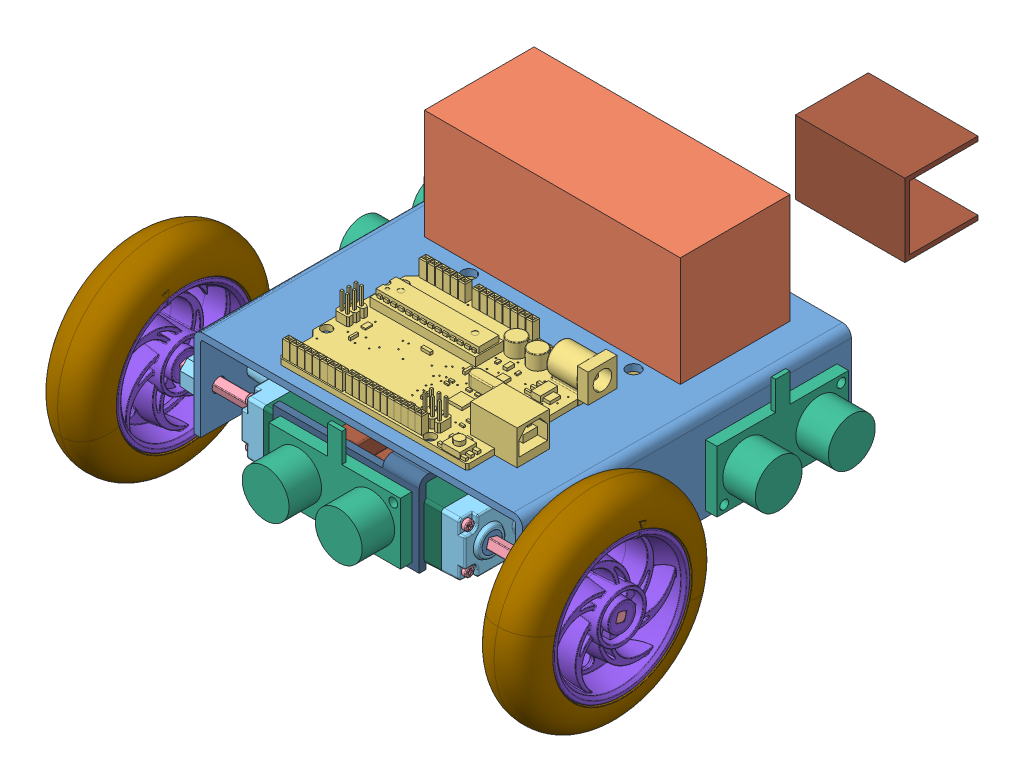
SolidWorks assembly mte380_Assy_02_minibot_01, configuration Default. Lengths in mm.
Overall size (174.7 100.24 233.03).
81 component instances, 29 part files, 49 mates.
Components (placement in the parent):
- mte380_02_frame_02-1: mte380_02_frame_02 [Default] at (-259.485 58.7791 95.25) size (114.15 31.84 114.3)
- mte380_02_package_01-1: mte380_02_package_01 [Default] at (-218.21 58.7791 46.8312) size (88.9 38.1 38.1)
- Arduino_Predeterminado-1: Arduino_Predeterminado [Default] at (-170.1744 58.7791 84.8989) x (-0.999979 0 0.006548) z (-0.006548 0 -0.999979) size (75 12 51.02)
- mte380_01_vex_motor_269-1: mte380_01_vex_motor_269 [Default] at (-184.6716 39.6426 96.8201) x (0 0 1) z (1 0 0) size (46.4 20.59 51.86)
  - SPPM206-0150BO-1: SPPM206-0150BO [Default] at (17.3 7.3 -1.5) x (1 0 0) z (0 -1 0) size (3.3 16.36 3.3)
  - 276-2181-003 Rev1-1: 276-2181-003 Rev1 [Default] at (0 0 -28) size (38.95 18.95 25.5)
  - 276-2177-019 Rev1-1: 276-2177-019 Rev1 [Default] at (-14.2702 0 -28) x (0.144195 -0.989549 0) z (0.989549 0.144195 0) size (6.3 15.8 6.3)
  - 276-2181-011 Rev1-1: 276-2181-011 Rev1 [Default] at (11.1298 0 -11) x (-1 0 0) z (0 1 0) size (11 4 11)
  - QFK-N30QAV-16068-1: QFK-N30QAV-16068 [Default] at (-12.9 0 -23) x (0 1 0) z (0 0 1) size (12 10 26.1)
  - SPPM143-0030BO-1: SPPM143-0030BO [Default] at (-12.9 4.25 -6) x (-1 0 0) z (0 1 0) size (2.4 6.08 2.4)
  - 276-2181-010 Rev1-1: 276-2181-010 Rev1 [Default] at (10.8763 0 -9.4) x (0.878827 0.47714 0) z (0 0 1) size (1.5 1.5 16)
  - 276-2181-001 Rev1-1: 276-2181-001 Rev1 [Default] at origin size (40 20 8.06)
  - 276-2181-006 Rev1-1: 276-2181-006 Rev1 [Default] at (10.8763 0 -1.05) x (-0.259931 -0.965627 0) z (0 0 1) size (14.22 14.25 6.9)
  - 276-2181-007 Rev1-1: 276-2181-007 Rev1 [Default] at (2.1533 -1.4937 -4.4) x (-0.202497 0.979283 0) z (0 0 1) size (14.22 14.25 14.9)
  - 276-2181-010 Rev1-2: 276-2181-010 Rev1 [Default] at (-5.7003 2.586 -9.4) size (1.5 1.5 16)
  - 276-2177-018 Rev1-1: 276-2177-018 Rev1 [Default] at (-18.5 0.1 2.5) x (0 1 0) z (1 0 0) size (6.4 4.2 8.9)
  - 276-2181-006 Rev1-2: 276-2181-006 Rev1 [Default] at (2.1533 -1.4937 2.75) x (-0.071378 0.997449 0) z (0 0 1) size (14.22 14.25 6.9)
  - 276-2181-002 Rev1-1: 276-2181-002 Rev1 [Default] at (0 0 -20) size (40 20 23)
  - 276-2181-009 Rev1-1: 276-2181-009 Rev1 [Default] at (2.1533 -1.4937 -26.5) size (1.5 1.5 33)
  - SPPM206-0150BO-2: SPPM206-0150BO [Default] at (-16.9263 6.9263 -18.5) x (-0.075705 0.99713 0) z (-0.99713 -0.075705 0) size (3.3 16.36 3.3)
  - 276-2181-011 Rev1-2: 276-2181-011 Rev1 [Default] at (11.1298 0 -24) x (-0.997622 -0.068917 0) z (-0.068917 0.997622 0) size (11 4 11)
  - 276-2177-019 Rev1-2: 276-2177-019 Rev1 [Default] at (-1.5702 0 -28) x (0.32391 -0.946088 0) z (0.946088 0.32391 0) size (6.3 15.8 6.3)
  - SPPM206-0150BO-3: SPPM206-0150BO [Default] at (-17.3 -7.3 -1.5) x (0.292947 -0.956129 0) z (-0.956129 -0.292947 0) size (3.3 16.36 3.3)
  - SPPM206-0150BO-4: SPPM206-0150BO [Default] at (16.9263 -6.9263 -18.5) x (0.149257 -0.988799 0) z (0.988799 0.149257 0) size (3.3 16.36 3.3)
  - SPPM206-0150BO-5: SPPM206-0150BO [Default] at (17.3 -7.3 -1.5) x (1 0 0) z (0 -1 0) size (3.3 16.36 3.3)
  - SPPM206-0150BO-6: SPPM206-0150BO [Default] at (-16.9263 -6.9263 -18.5) x (-0.049887 0.998755 0) z (-0.998755 -0.049887 0) size (3.3 16.36 3.3)
  - SPPM206-0150BO-7: SPPM206-0150BO [Default] at (-17.3 7.3 -1.5) x (-0.963198 0.268794 0) z (0.268794 0.963198 0) size (3.3 16.36 3.3)
  - SPPM206-0150BO-8: SPPM206-0150BO [Default] at (16.9263 6.9263 -18.5) x (0.906825 0.421508 0) z (-0.421508 0.906825 0) size (3.3 16.36 3.3)
  - SPPM143-0030BO-2: SPPM143-0030BO [Default] at (-12.9 -4.25 -6) x (-0.988208 -0.153116 0) z (-0.153116 0.988208 0) size (2.4 6.08 2.4)
  - 276-2181-004 Rev1-1: 276-2181-004 Rev1 [Default] at (-12.9 0 -0.1) x (0.94341 -0.331628 0) z (0 0 -1) size (5.17 5.4 3)
  - 276-2181-005 Rev1-1: 276-2181-005 Rev1 [Default] at (-5.7003 2.586 -0.05) x (0.460478 -0.887671 0) z (0 0 1) size (11.88 11.88 5.9)
  - 276-2181-008 Rev1_276-2181-008g-1: 276-2181-008 Rev1_276-2181-008g [Default] at (11.1298 0 -14.5) x (0.267616 -0.963526 0) z (0 0 -1) size (13.83 13.88 17.3)
  - 276-2181-012 Rev1-1: 276-2181-012 Rev1 [Default] at (-12.9 0 -24) size (13.6 13 1)
- mte380_01_vex_motor_269-2: mte380_01_vex_motor_269 [Default] at (-162.8484 39.6426 96.8202) x (0 0 1) z (-1 0 0) size (46.4 20.59 51.86)
  - SPPM206-0150BO-1: SPPM206-0150BO [Default] at (17.3 7.3 -1.5) x (1 0 0) z (0 -1 0) size (3.3 16.36 3.3)
  - 276-2181-003 Rev1-1: 276-2181-003 Rev1 [Default] at (0 0 -28) size (38.95 18.95 25.5)
  - 276-2177-019 Rev1-1: 276-2177-019 Rev1 [Default] at (-14.2702 0 -28) x (0.144195 -0.989549 0) z (0.989549 0.144195 0) size (6.3 15.8 6.3)
  - 276-2181-011 Rev1-1: 276-2181-011 Rev1 [Default] at (11.1298 0 -11) x (-1 0 0) z (0 1 0) size (11 4 11)
  - QFK-N30QAV-16068-1: QFK-N30QAV-16068 [Default] at (-12.9 0 -23) x (0 1 0) z (0 0 1) size (12 10 26.1)
  - SPPM143-0030BO-1: SPPM143-0030BO [Default] at (-12.9 4.25 -6) x (-1 0 0) z (0 1 0) size (2.4 6.08 2.4)
  - 276-2181-010 Rev1-1: 276-2181-010 Rev1 [Default] at (10.8763 0 -9.4) x (0.878827 0.47714 0) z (0 0 1) size (1.5 1.5 16)
  - 276-2181-001 Rev1-1: 276-2181-001 Rev1 [Default] at origin size (40 20 8.06)
  - 276-2181-006 Rev1-1: 276-2181-006 Rev1 [Default] at (10.8763 0 -1.05) x (-0.259931 -0.965627 0) z (0 0 1) size (14.22 14.25 6.9)
  - 276-2181-007 Rev1-1: 276-2181-007 Rev1 [Default] at (2.1533 -1.4937 -4.4) x (-0.202497 0.979283 0) z (0 0 1) size (14.22 14.25 14.9)
  - 276-2181-010 Rev1-2: 276-2181-010 Rev1 [Default] at (-5.7003 2.586 -9.4) size (1.5 1.5 16)
  - 276-2177-018 Rev1-1: 276-2177-018 Rev1 [Default] at (-18.5 0.1 2.5) x (0 1 0) z (1 0 0) size (6.4 4.2 8.9)
  - 276-2181-006 Rev1-2: 276-2181-006 Rev1 [Default] at (2.1533 -1.4937 2.75) x (-0.071378 0.997449 0) z (0 0 1) size (14.22 14.25 6.9)
  - 276-2181-002 Rev1-1: 276-2181-002 Rev1 [Default] at (0 0 -20) size (40 20 23)
  - 276-2181-009 Rev1-1: 276-2181-009 Rev1 [Default] at (2.1533 -1.4937 -26.5) size (1.5 1.5 33)
  - SPPM206-0150BO-2: SPPM206-0150BO [Default] at (-16.9263 6.9263 -18.5) x (-0.075705 0.99713 0) z (-0.99713 -0.075705 0) size (3.3 16.36 3.3)
  - 276-2181-011 Rev1-2: 276-2181-011 Rev1 [Default] at (11.1298 0 -24) x (-0.997622 -0.068917 0) z (-0.068917 0.997622 0) size (11 4 11)
  - 276-2177-019 Rev1-2: 276-2177-019 Rev1 [Default] at (-1.5702 0 -28) x (0.32391 -0.946088 0) z (0.946088 0.32391 0) size (6.3 15.8 6.3)
  - SPPM206-0150BO-3: SPPM206-0150BO [Default] at (-17.3 -7.3 -1.5) x (0.292947 -0.956129 0) z (-0.956129 -0.292947 0) size (3.3 16.36 3.3)
  - SPPM206-0150BO-4: SPPM206-0150BO [Default] at (16.9263 -6.9263 -18.5) x (0.149257 -0.988799 0) z (0.988799 0.149257 0) size (3.3 16.36 3.3)
  - SPPM206-0150BO-5: SPPM206-0150BO [Default] at (17.3 -7.3 -1.5) x (1 0 0) z (0 -1 0) size (3.3 16.36 3.3)
  - SPPM206-0150BO-6: SPPM206-0150BO [Default] at (-16.9263 -6.9263 -18.5) x (-0.049887 0.998755 0) z (-0.998755 -0.049887 0) size (3.3 16.36 3.3)
  - SPPM206-0150BO-7: SPPM206-0150BO [Default] at (-17.3 7.3 -1.5) x (-0.963198 0.268794 0) z (0.268794 0.963198 0) size (3.3 16.36 3.3)
  - SPPM206-0150BO-8: SPPM206-0150BO [Default] at (16.9263 6.9263 -18.5) x (0.906825 0.421508 0) z (-0.421508 0.906825 0) size (3.3 16.36 3.3)
  - SPPM143-0030BO-2: SPPM143-0030BO [Default] at (-12.9 -4.25 -6) x (-0.988208 -0.153116 0) z (-0.153116 0.988208 0) size (2.4 6.08 2.4)
  - 276-2181-004 Rev1-1: 276-2181-004 Rev1 [Default] at (-12.9 0 -0.1) x (0.94341 -0.331628 0) z (0 0 -1) size (5.17 5.4 3)
  - 276-2181-005 Rev1-1: 276-2181-005 Rev1 [Default] at (-5.7003 2.586 -0.05) x (0.460478 -0.887671 0) z (0 0 1) size (11.88 11.88 5.9)
  - 276-2181-008 Rev1_276-2181-008g-1: 276-2181-008 Rev1_276-2181-008g [Default] at (11.1298 0 -14.5) x (0.267616 -0.963526 0) z (0 0 -1) size (13.83 13.88 17.3)
  - 276-2181-012 Rev1-1: 276-2181-012 Rev1 [Default] at (-12.9 0 -24) size (13.6 13 1)
- mte380_01_reedy_battery_pack-1: mte380_01_reedy_battery_pack [Default] at (-130.58 56.4169 39.2112) x (-1 0 0) z (0 0 1) size (86.36 16.51 30.48)
- mte380_01_vex_shaft_2-1: mte380_01_vex_shaft_2 [Default] at (-233.3716 39.6603 107.9813) x (0 0.267617 -0.963525) z (1 0 0) size (3.17 3.17 51.01)
- mte380_01_vex_flat_bearing-1: mte380_01_vex_flat_bearing [Default] at (-27.71 26.9427 121.666) x (-1 0 0) z (0 -1 0) size (7.04 35.56 10.16)
- mte380_01_ultrasonic-1: mte380_01_ultrasonic [Default] at (-116.6862 50.3977 5) x (0 0 1) z (0 1 0) size (45.7 15.3 31.3)
- mte380_vex_wheel-1: mte380_vex_wheel [Default] at (-95.2912 20.4764 97.5479) x (0 -0.267616 -0.963526) z (1 0 0) size (69.86 69.86 23.08)
  - SMALL-WHEEL-RIM-1: SMALL-WHEEL-RIM [Default] at (-15.1515 15.6838 -2.6601) size (61.43 61.43 9.25)
  - SMALL-WHEEL-HUB-1: SMALL-WHEEL-HUB [Default] at (-15.1515 15.6838 -2.6601) size (61.36 61.43 23.08)
  - SMALL-WHEEL-TIRE-1: SMALL-WHEEL-TIRE [Default] at (-15.1515 15.6838 -2.6601) x (1 0 0) z (0 -1 0) size (69.86 19.99 69.86)
- mte380_02_front_ultrasonic_mount_01-1: mte380_02_front_ultrasonic_mount_01 [Default] at (-199.4633 27.9181 118.1983) x (1 0 0) z (0 -1 0) size (50.8 63.59 28.5)
- mte380_01_ultrasonic-2: mte380_01_ultrasonic [Default] at (-151.1833 51.2461 118.1983) x (-1 0 0) z (0 1 0) size (45.7 15.3 31.3)
- mte380_01_vex_flat_bearing-2: mte380_01_vex_flat_bearing [Default] at (-319.81 26.9427 68.834) x (1 0 0) z (0 -1 0) size (7.04 35.56 10.16)
- mte380_vex_wheel-2: mte380_vex_wheel [Default] at (-246.9086 28.6208 89.216) x (0 0.267617 -0.963525) z (1 0 0) size (69.86 69.86 23.08)
  - SMALL-WHEEL-RIM-1: SMALL-WHEEL-RIM [Default] at (-15.1515 15.6838 -2.6601) size (61.43 61.43 9.25)
  - SMALL-WHEEL-HUB-1: SMALL-WHEEL-HUB [Default] at (-15.1515 15.6838 -2.6601) size (61.36 61.43 23.08)
  - SMALL-WHEEL-TIRE-1: SMALL-WHEEL-TIRE [Default] at (-15.1515 15.6838 -2.6601) x (1 0 0) z (0 -1 0) size (69.86 19.99 69.86)
- mte380_01_vex_shaft_2-2: mte380_01_vex_shaft_2 [Default] at (-114.1484 39.6603 107.9187) x (0 -0.267616 -0.963526) z (1 0 0) size (3.17 3.17 51.01)
- mte380_01_ultrasonic-3: mte380_01_ultrasonic [Default] at (-230.8338 50.3977 50.7) x (0 0 -1) z (0 1 0) size (45.7 15.3 31.3)
- mte380_02_caster_ball_mount_01-1: mte380_02_caster_ball_mount_01 [Default] at (-192.81 56.4169 -82.0137) x (0 0 -1) z (0 -1 0) size (25.4 38.1 25.4)
Mates (geometry in assembly coordinates):
- Concentric1: concentric anti-aligned: cylinder of mte380_02_frame_02-1 through (-230.8338 39.6427 107.95) axis (1 0 0) radius 2.3813; cylinder of mte380_01_vex_flat_bearing-2 through (-237.1838 39.6427 107.95) axis (-1 0 0) radius 2.1209
- Concentric2: concentric anti-aligned: cylinder of mte380_02_frame_02-1 through (-230.8338 39.6427 82.55) axis (1 0 0) radius 2.3813; cylinder of mte380_01_vex_flat_bearing-2 through (-237.1838 39.6427 82.55) axis (-1 0 0) radius 2.1209
- Coincident1: coincident anti-aligned: plane of mte380_02_frame_02-1 through (-230.8338 26.9427 95.25) normal (-1 0 0); plane of mte380_01_vex_flat_bearing-2 through (-230.8338 26.9427 68.834) normal (1 0 0)
- Coincident2: coincident anti-aligned: plane of mte380_01_vex_shaft_2-1 through (-207.9716 38.5556 106.0268) normal (0 0.267617 -0.963525); plane of mte380_vex_wheel-2/SMALL-WHEEL-HUB-1 through (-238.1387 38.5556 106.0268) normal (0 -0.267617 0.963525)
- Coincident3: coincident anti-aligned: plane of mte380_01_vex_shaft_2-1 through (-207.9716 37.7059 109.086) normal (0 -0.963525 -0.267617); plane of mte380_vex_wheel-2/SMALL-WHEEL-HUB-1 through (-238.1387 37.6925 109.1342) normal (0 0.963525 0.267617)
- Tangent1: tangent: plane of mte380_01_vex_shaft_2-1 through (-258.7716 40.7651 109.9357) normal (-1 0 0); face of mte380_vex_wheel-2/SMALL-WHEEL-HUB-1
- Coincident11: coincident anti-aligned: plane of mte380_02_frame_02-1 through (-259.485 58.7791 95.25) normal (0 1 0); plane of mte380_02_package_01-1 through (-129.31 58.7791 46.8312) normal (0 -1 0)
- Width1: width aligned: plane of mte380_02_package_01-1 through (-129.31 58.7791 46.8312) normal (1 0 0); plane of mte380_02_package_01-1 through (-218.21 58.7791 46.8312) normal (-1 0 0); plane of mte380_02_frame_02-1 through (-116.6862 198.3927 95.25) normal (1 0 0); plane of mte380_02_frame_02-1 through (-230.8338 26.9427 95.25) normal (-1 0 0)
- Width2: width anti-aligned: plane of mte380_01_reedy_battery_pack-1 through (-216.94 56.4169 39.2112) normal (-1 0 0); plane of mte380_01_reedy_battery_pack-1 through (-130.58 56.4169 39.2112) normal (1 0 0); plane of mte380_02_frame_02-1 through (-228.4716 26.9427 95.25) normal (1 0 0); plane of mte380_02_frame_02-1 through (-119.0484 198.3927 95.25) normal (-1 0 0)
- Coincident12: coincident anti-aligned: plane of mte380_02_frame_02-1 through (-259.485 56.4169 95.25) normal (0 -1 0); plane of mte380_01_reedy_battery_pack-1 through (-216.94 56.4169 39.2112) normal (0 1 0)
- Concentric3: concentric aligned: cylinder of mte380_02_frame_02-1 through (-155.0148 26.9417 107.95) axis (0 1 0) radius 1.7996; cylinder of Arduino_Predeterminado-1 through (-155.0141 50.2791 107.9506) axis (0 1 0) radius 1.8
- Concentric4: concentric anti-aligned: circle of mte380_02_frame_02-1; circle of Arduino_Predeterminado-1
- Coincident13: coincident anti-aligned: plane of mte380_02_frame_02-1 through (-259.485 58.7791 95.25) normal (0 1 0); plane of Arduino_Predeterminado-1 through (-170.1744 58.7791 84.8989) normal (0 -1 0)
- Coincident14: coincident anti-aligned: plane of mte380_01_vex_motor_269-1/276-2181-008 Rev1_276-2181-008g-1 through (-207.9716 37.6569 109.0724) normal (0 0.267617 -0.963525); plane of mte380_01_vex_shaft_2-1 through (-207.9716 37.7059 109.086) normal (0 -0.267617 0.963525)
- Coincident15: coincident anti-aligned: plane of mte380_01_vex_motor_269-1/276-2181-008 Rev1_276-2181-008g-1 through (-207.9716 40.7651 109.9357) normal (0 -0.963525 -0.267617); plane of mte380_01_vex_shaft_2-1 through (-207.9716 40.7651 109.9357) normal (0 0.963525 0.267617)
- Coincident16: coincident anti-aligned: plane of mte380_01_vex_motor_269-1/276-2181-008 Rev1_276-2181-008g-1 through (-207.9716 41.6284 106.8276) normal (-1 0 0); plane of mte380_01_vex_shaft_2-1 through (-207.9716 40.7651 109.9357) normal (1 0 0)
- Concentric5: concentric aligned: cylinder of mte380_01_vex_motor_269-1/276-2177-019 Rev1-1 through (-228.4716 39.6427 82.55) axis (-1 0 0) radius 1.3526; circle of mte380_01_vex_flat_bearing-2
- Concentric6: concentric anti-aligned: circle of Arduino_Predeterminado-1; circle of mte380_02_front_ultrasonic_mount_01-1
- Coincident17: coincident anti-aligned: plane of mte380_02_frame_02-1 through (-259.485 56.4169 95.25) normal (0 -1 0); plane of mte380_02_front_ultrasonic_mount_01-1 through (-199.4633 56.4169 143.5118) normal (0 1 0)
- Coincident19: coincident anti-aligned: plane of mte380_02_front_ultrasonic_mount_01-1 through (-199.4633 27.9181 118.1983) normal (0 0 1); plane of mte380_01_ultrasonic-2 through (-151.1833 51.2461 118.1983) normal (0 0 -1)
- Concentric8: concentric anti-aligned: circle of mte380_02_front_ultrasonic_mount_01-1; circle of mte380_01_ultrasonic-2
- Concentric9: concentric anti-aligned: cylinder of mte380_02_front_ultrasonic_mount_01-1 through (-194.3833 32.4461 54.6108) axis (0 0 1) radius 1.55; cylinder of mte380_01_ultrasonic-2 through (-194.3833 32.4461 122.1983) axis (0 0 -1) radius 1.55
- Concentric10: concentric aligned: cylinder of mte380_01_vex_motor_269-1/276-2177-019 Rev1-2 through (-228.4716 39.6426 95.25) axis (-1 0 0) radius 1.3526; cylinder of mte380_01_vex_flat_bearing-2 through (-237.1838 39.6426 95.25) axis (-1 0 0) radius 2.1209
- Coincident23: coincident anti-aligned: plane of mte380_02_frame_02-1 through (-228.4716 26.9427 95.25) normal (1 0 0); plane of mte380_01_vex_motor_269-1/276-2177-019 Rev1-1 through (-228.4716 39.6427 82.55) normal (-1 0 0)
- Parallel3: parallel: plane of mte380_02_frame_02-1 through (-259.485 56.4169 114.3) normal (0 0 1); line of mte380_02_front_ultrasonic_mount_01-1 through (-161.3633 53.3181 115.8361) axis (-1 0 0)
- Concentric12: concentric aligned: circle of mte380_02_frame_02-1; cylinder of mte380_01_vex_flat_bearing-1 through (-110.3362 39.6427 82.55) axis (1 0 0) radius 2.1209
- Concentric13: concentric aligned: circle of mte380_02_frame_02-1; circle of mte380_01_vex_flat_bearing-1
- Coincident26: coincident anti-aligned: plane of mte380_02_frame_02-1 through (-116.6862 198.3927 95.25) normal (1 0 0); plane of mte380_01_vex_flat_bearing-1 through (-116.6862 26.9427 121.666) normal (-1 0 0)
- Concentric15: concentric anti-aligned: circle of mte380_01_vex_motor_269-2/276-2177-019 Rev1-1; circle of mte380_01_vex_flat_bearing-1
- Concentric16: concentric anti-aligned: circle of mte380_01_vex_motor_269-2/276-2177-019 Rev1-2; circle of mte380_01_vex_flat_bearing-1
- Coincident27: coincident anti-aligned: plane of mte380_02_frame_02-1 through (-119.0484 198.3927 95.25) normal (-1 0 0); circle of mte380_01_vex_motor_269-2/276-2177-019 Rev1-1
- Coincident28: coincident anti-aligned: plane of mte380_01_vex_motor_269-2/276-2181-008 Rev1_276-2181-008g-1 through (-139.5484 41.6283 109.0724) normal (0 -0.963526 0.267616); plane of mte380_01_vex_shaft_2-2 through (-88.7484 41.6148 109.0235) normal (0 0.963526 -0.267616)
- Coincident29: coincident anti-aligned: plane of mte380_01_vex_motor_269-2/276-2181-008 Rev1_276-2181-008g-1 through (-139.5484 40.7651 105.9643) normal (0 0.267616 0.963526); plane of mte380_01_vex_shaft_2-2 through (-88.7484 37.7059 106.814) normal (0 -0.267616 -0.963526)
- Coincident30: coincident anti-aligned: plane of mte380_01_vex_motor_269-2/276-2181-008 Rev1_276-2181-008g-1 through (-139.5484 37.6569 106.8276) normal (1 0 0); plane of mte380_01_vex_shaft_2-2 through (-139.5484 41.6148 109.0235) normal (-1 0 0)
- Coincident31: coincident anti-aligned: plane of mte380_vex_wheel-1/SMALL-WHEEL-HUB-1 through (-86.5213 40.7651 105.9643) normal (0 -0.963526 0.267616); plane of mte380_01_vex_shaft_2-2 through (-88.7484 41.6148 109.0235) normal (0 0.963526 -0.267616)
- Coincident32: coincident anti-aligned: plane of ? through (-86.5213 37.6577 106.8274) normal (0 0.267616 0.963526); plane of mte380_01_vex_shaft_2-2 through (-88.7484 37.7059 106.814) normal (0 -0.267616 -0.963526)
- Tangent2: tangent: face of ?; plane of mte380_01_vex_shaft_2-2 through (-88.7484 41.6148 109.0235) normal (1 0 0)
- Concentric17: concentric anti-aligned: circle of mte380_02_frame_02-1; circle of mte380_01_ultrasonic-1
- Concentric18: concentric anti-aligned: circle of mte380_02_frame_02-1; circle of mte380_01_ultrasonic-1
- Coincident35: coincident anti-aligned: plane of mte380_02_frame_02-1 through (-116.6862 198.3927 95.25) normal (1 0 0); plane of mte380_01_ultrasonic-1 through (-116.6862 50.3977 5) normal (-1 0 0)
- Tangent3: tangent: circle of mte380_02_frame_02-1; plane of mte380_02_package_01-1 through (-129.31 58.7791 8.7312) normal (0 0 -1)
- Tangent4: tangent: circle of mte380_02_frame_02-1; plane of mte380_01_reedy_battery_pack-1 through (-216.94 56.4169 8.7312) normal (0 0 -1)
- Concentric21: concentric anti-aligned: circle of mte380_02_frame_02-1; cylinder of mte380_01_ultrasonic-3 through (-234.8338 31.5977 7.5) axis (1 0 0) radius 1.55
- Coincident42: coincident anti-aligned: plane of mte380_02_frame_02-1 through (-230.8338 26.9427 95.25) normal (-1 0 0); plane of mte380_01_ultrasonic-3 through (-230.8338 50.3977 50.7) normal (1 0 0)
- Concentric22: concentric anti-aligned: circle of mte380_02_frame_02-1; circle of mte380_01_ultrasonic-3
- Parallel4: parallel anti-aligned: plane of mte380_02_frame_02-1 through (-259.485 56.4169 95.25) normal (0 -1 0); plane of assembly through (0 0 0) normal (0 1 0)
- Coincident44: coincident anti-aligned: plane of mte380_02_frame_02-1 through (-259.485 56.4169 0) normal (0 0 -1); plane of assembly through (0 0 0) normal (0 0 1)
- Coincident45: coincident anti-aligned: plane of mte380_02_frame_02-1 through (-259.485 56.4169 95.25) normal (0 -1 0); plane of mte380_02_caster_ball_mount_01-1 through (-154.71 56.4169 -82.0137) normal (0 1 0)
- Width3: width anti-aligned: plane of mte380_02_caster_ball_mount_01-1 through (-154.71 56.4169 -82.0137) normal (1 0 0); plane of mte380_02_caster_ball_mount_01-1 through (-192.81 56.4169 -82.0137) normal (-1 0 0); plane of mte380_02_frame_02-1 through (-119.0484 198.3927 95.25) normal (-1 0 0); plane of mte380_02_frame_02-1 through (-228.4716 26.9427 95.25) normal (1 0 0)
